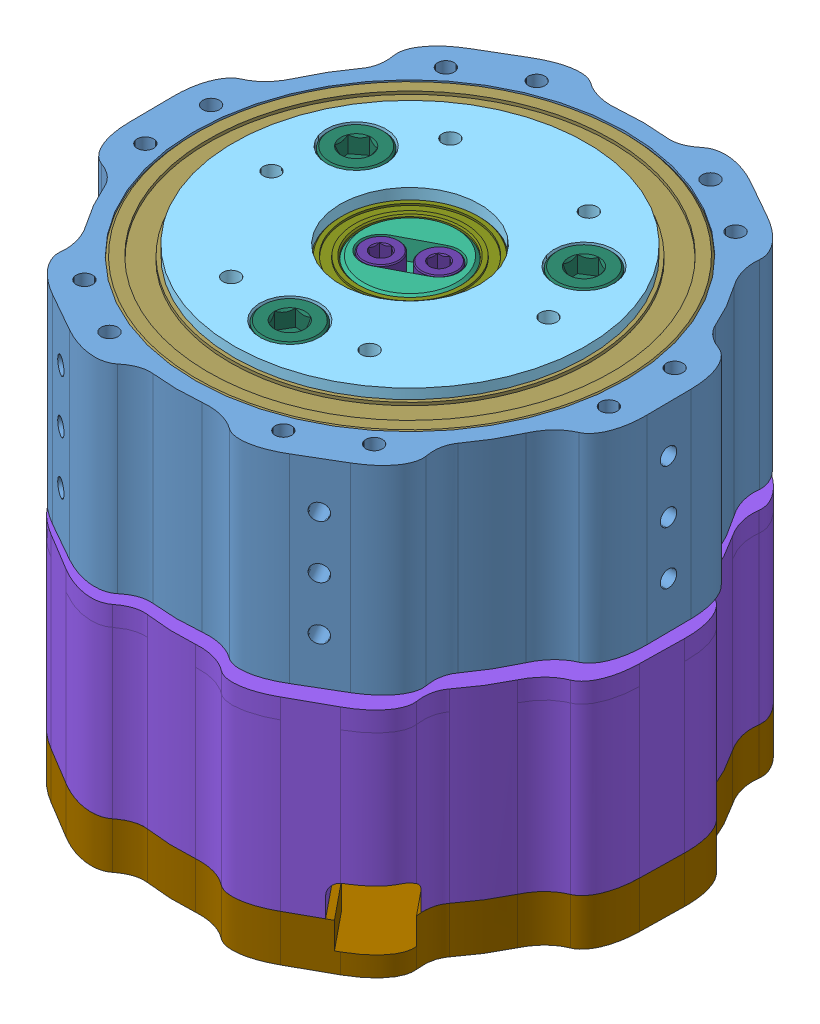
SolidWorks assembly LTRPT-0001-0000-00 (Assembly), configuration Resin 3D Print Config. Lengths in mm.
Overall size (104.8 68.77 105.06).
52 component instances, 20 part files, 70 mates.
Components (placement in the parent):
- LTRPT-0001-0001-00-1: LTRPT-0001-0001-00 [Pinless] at (0.2542 76.0347 0.3117) x (-0.492208 0 0.870478) z (-0.870478 0 -0.492208)
- LTRPT-0001-0002-00-1: LTRPT-0001-0002-00 [Default] at (0.2542 73.0347 0.3117) x (0.886253 0 -0.463201) z (0.463201 0 0.886253) (hidden)
- LTRPT-0001-0003-00-1: LTRPT-0001-0003-00 [Default] at (-0.632 82.5347 0.7749) x (-0.034899 0 -0.999391) z (0.999391 0 -0.034899)
- LTRPT-0001-0004-00-1: LTRPT-0001-0004-00 [Default] at (1.1405 91.5347 -0.1515) x (0.121869 0 -0.992546) z (0.992546 0 0.121869)
- LTRPT-0001-0005-00-1: LTRPT-0001-0005-00 [Default] at (0.2542 76.0347 0.3117) x (-0.998988 0 0.044987) z (-0.044987 0 -0.998988)
- LTRPT-0001-0006-00-1: LTRPT-0001-0006-00 [Default] at (0.2542 100.0347 0.3117) x (0.538454 0 0.842655) z (-0.842655 0 0.538454)
- LTRPT-0001-0007-00-1: LTRPT-0001-0007-00 [Default] at (1.1405 91.0347 -0.1515) x (-0.886253 0 0.463201) z (-0.463201 0 -0.886253)
- LTRPT-0001-0008-00-1: LTRPT-0001-0008-00 [Default] at (0.2542 76.0347 0.3117) x (-0.886253 0 0.463201) z (-0.463201 0 -0.886253)
- LTRPT-0001-0006-01-1: LTRPT-0001-0006-01 [Default] at (0.2542 100.0347 0.3117) x (0.538454 0 0.842655) z (-0.842655 0 0.538454) (hidden)
- LTRPT-0001-0009-00-1: LTRPT-0001-0009-00 [Pinless] at (0.2542 46.0347 0.3117) x (0.999837 0 0.018067) z (-0.018067 0 0.999837) size (77.35 28.07 76.65)
- LTRPT-0001-0010-01-1: LTRPT-0001-0010-01 [Default] at (0.2542 42.0347 0.3117) x (-0.999837 0 -0.018067) z (0 -1 0) size (77.35 73.91 7.07)
- LTRPT-0001-0011-00-1: LTRPT-0001-0011-00 [Default] at (0.2542 71.3347 0.3117) x (0.984702 0 0.174247) z (0 1 0) size (19.5 19.5 4.5)
- LTRPT-0001-0012-00-1: LTRPT-0001-0012-00 [Default] at (14.0653 40.3347 -2.5639) x (-0.953415 0 -0.301661) z (0 -1 0) size (77.35 73.91 4.57) (hidden)
- GARTT ML5008 330KV-1: GARTT ML5008 330KV [Default] at (0.2542 46.0347 0.3117) x (0.984702 0 0.174247) z (-0.174247 0 0.984702)
- 6656K229_Ultra-Thin Ball Bearing-1: 6656K229_Ultra-Thin Ball Bearing [6656K229] at (0.2542 102.5347 0.3117) x (0.90683 0 0.421496) z (0 1 0)
- 6656K229_Ultra-Thin Ball Bearing-2: 6656K229_Ultra-Thin Ball Bearing [6656K229] at (0.2542 79.5347 0.3117) x (0.89109 0 -0.453826) z (0 1 0)
- 5x25mm Dowel Pin-1: 5x25mm Dowel Pin [Default] at (-15.7562 78.0347 10.5424) x (-0.5743 0 0.818645) z (-0.818645 0 -0.5743)
- 5x25mm Dowel Pin-5: 5x25mm Dowel Pin [Default] at (17.1194 78.0347 9.0619) x (-0.146093 0 -0.989271) z (0.989271 0 -0.146093)
- 5x25mm Dowel Pin-6: 5x25mm Dowel Pin [Default] at (-0.6005 78.0347 -18.669) x (0.11323 0 -0.993569) z (0.993569 0 0.11323)
- MR95ZZ-1: MR95ZZ [Predeterminado] at (-15.7562 91.5347 10.5424) x (0.985719 0 -0.168399) z (0 1 0)
- MR95ZZ-2: MR95ZZ [Predeterminado] at (-15.7562 87.5347 10.5424) x (1 0 0.000798) z (0 1 0)
- MR95ZZ-3: MR95ZZ [Predeterminado] at (-15.7562 83.5347 10.5424) x (-0.502758 0 0.864427) z (0 1 0)
- MR95ZZ-4: MR95ZZ [Predeterminado] at (-15.7562 95.5347 10.5424) x (-0.758179 0 0.652046) z (0 1 0)
- 91290A252_Alloy Steel Socket Head Screw-1: 91290A252_Alloy Steel Socket Head Screw [Low Poly] at (16.2647 92.5347 -9.9189) x (0.999255 0 -0.038584) z (0 1 0)
- 91290A252_Alloy Steel Socket Head Screw-2: 91290A252_Alloy Steel Socket Head Screw [Low Poly] at (1.109 92.5347 19.2925) x (0.015336 0 -0.999882) z (0 1 0)
- 91290A252_Alloy Steel Socket Head Screw-3: 91290A252_Alloy Steel Socket Head Screw [Low Poly] at (-16.611 92.5347 -8.4384) x (-0.383105 0 0.923705) z (0 1 0)
- 6656K182_Ultra-Thin Ball Bearing-1: 6656K182_Ultra-Thin Ball Bearing [6656K182] at (0 79.0347 0) x (-0.858071 0 -0.513532) z (0 1 0)
- 6656K182_Ultra-Thin Ball Bearing-2: 6656K182_Ultra-Thin Ball Bearing [6656K182] at (0.2542 104.0347 0.3117) x (0.999223 0 -0.039404) z (0 1 0)
- 6656K182_Ultra-Thin Ball Bearing-3: 6656K182_Ultra-Thin Ball Bearing [6656K182] at (-0.632 88.0347 0.7749) x (0.999223 0 -0.039404) z (0 1 0)
- 6656K182_Ultra-Thin Ball Bearing-4: 6656K182_Ultra-Thin Ball Bearing [6656K182] at (1.1405 94.5347 -0.1515) x (0.999223 0 -0.039404) z (0 1 0)
- 91290A130_Black-Oxide Alloy Steel Socket Head Screw-1: 91290A130_Black-Oxide Alloy Steel Socket Head Screw [Low Poly] at (3.1345 89.5347 -1.1937) x (0.78846 0 0.615086) z (0 1 0)
- 91290A130_Black-Oxide Alloy Steel Socket Head Screw-2: 91290A130_Black-Oxide Alloy Steel Socket Head Screw [Low Poly] at (-2.6261 89.5347 1.8171) x (0.78846 0 0.615086) z (0 1 0)
- MR95ZZ-9: MR95ZZ [Predeterminado] at (-16.611 95.5347 -8.4384) x (-0.943778 0 -0.330579) z (0 1 0)
- MR95ZZ-10: MR95ZZ [Predeterminado] at (-0.6005 95.5347 -18.669) x (-0.185599 0 -0.982626) z (0 1 0)
- MR95ZZ-11: MR95ZZ [Predeterminado] at (16.2647 95.5347 -9.9189) x (0.758179 0 -0.652046) z (0 1 0)
- MR95ZZ-12: MR95ZZ [Predeterminado] at (17.1194 95.5347 9.0619) x (0.943778 0 0.330579) z (0 1 0)
- MR95ZZ-13: MR95ZZ [Predeterminado] at (1.109 95.5347 19.2925) x (0.185599 0 0.982626) z (0 1 0)
- MR95ZZ-14: MR95ZZ [Predeterminado] at (-16.611 91.5347 -8.4384) x (0.638697 0 0.769458) z (0 1 0)
- MR95ZZ-15: MR95ZZ [Predeterminado] at (-0.6005 91.5347 -18.669) x (-0.347022 0 0.937857) z (0 1 0)
- MR95ZZ-16: MR95ZZ [Predeterminado] at (16.2647 91.5347 -9.9189) x (-0.985719 0 0.168399) z (0 1 0)
- MR95ZZ-17: MR95ZZ [Predeterminado] at (17.1194 91.5347 9.0619) x (-0.638697 0 -0.769458) z (0 1 0)
- MR95ZZ-18: MR95ZZ [Predeterminado] at (1.109 91.5347 19.2925) x (0.347022 0 -0.937857) z (0 1 0)
- MR95ZZ-19: MR95ZZ [Predeterminado] at (-16.611 87.5347 -8.4384) x (0.499309 0 0.866424) z (0 1 0)
- MR95ZZ-20: MR95ZZ [Predeterminado] at (-0.6005 87.5347 -18.669) x (-0.500691 0 0.865626) z (0 1 0)
- MR95ZZ-21: MR95ZZ [Predeterminado] at (16.2647 87.5347 -9.9189) x (-1 0 -0.000798) z (0 1 0)
- MR95ZZ-22: MR95ZZ [Predeterminado] at (17.1194 87.5347 9.0619) x (-0.499309 0 -0.866424) z (0 1 0)
- MR95ZZ-23: MR95ZZ [Predeterminado] at (1.109 87.5347 19.2925) x (0.500691 0 -0.865626) z (0 1 0)
- MR95ZZ-24: MR95ZZ [Predeterminado] at (-16.611 83.5347 -8.4384) x (-0.999995 0 -0.003188) z (0 1 0)
- MR95ZZ-25: MR95ZZ [Predeterminado] at (-0.6005 83.5347 -18.669) x (-0.497237 0 -0.867615) z (0 1 0)
- MR95ZZ-26: MR95ZZ [Predeterminado] at (16.2647 83.5347 -9.9189) x (0.502758 0 -0.864427) z (0 1 0)
- MR95ZZ-27: MR95ZZ [Predeterminado] at (17.1194 83.5347 9.0619) x (0.999995 0 0.003188) z (0 1 0)
- MR95ZZ-28: MR95ZZ [Predeterminado] at (1.109 83.5347 19.2925) x (0.497237 0 0.867615) z (0 1 0)
Mates (geometry in assembly coordinates):
- Concentric5: concentric aligned: cylinder of Actuator Body-1 through (0.2542 0 0.3117) axis (0 -1 0) radius 35; cylinder of LTRPT-0001-0001-00-1 through (0.2542 84.0347 0.3117) axis (0 -1 0) radius 35
- Angle2: planar angle = 0.034907 rad anti-aligned: plane of LTRPT-0001-0003-00-1 through (-0.632 82.5347 0.7749) normal (-0.034899 0 -0.999391)
- Angle3: planar angle = 0.15708 rad aligned: plane of LTRPT-0001-0003-00-1 through (-0.632 82.5347 0.7749) normal (-0.034899 0 -0.999391); plane of LTRPT-0001-0004-00-1 through (1.1405 91.5347 -0.1515) normal (0.121869 0 -0.992546)
- Coincident27: coordinate: point of Eccentric Bottom Bearing Housing-1
- Concentric28: concentric aligned: cylinder of LTRPT-0001-0003-00-1 through (-0.632 90.5347 0.7749) axis (0 -1 0) radius 10.4; cylinder of LTRPT-0001-0008-00-1 through (-0.632 91.0347 0.7749) axis (0 -1 0) radius 7.5
- Coincident36: coincident aligned: plane of LTRPT-0001-0001-00-1 through (0.2542 84.0347 0.3117) normal (0 -1 0); plane of LTRPT-0001-0008-00-1 through (-0.632 84.0347 0.7749) normal (0 -1 0)
- Coincident37: coincident aligned: plane of LTRPT-0001-0001-00-1 through (0.2542 76.0347 0.3117) normal (0 -1 0); plane of 6656K229_Ultra-Thin Ball Bearing-2 through (-14.3363 76.0347 -28.3368) normal (0 -1 0)
- Coincident38: coincident aligned: plane of LTRPT-0001-0001-00-1 through (0.2542 106.0347 0.3117) normal (0 1 0); plane of 6656K229_Ultra-Thin Ball Bearing-1 through (13.8053 106.0347 -28.8429) normal (0 1 0)
- Concentric33: concentric anti-aligned: cylinder of LTRPT-0001-0006-00-1 through (-15.7562 100.0347 10.5424) axis (0 1 0) radius 2.5; cylinder of 5x25mm Dowel Pin-1 through (-15.7562 103.0347 10.5424) axis (0 -1 0) radius 2.5
- Concentric35: concentric anti-aligned: cylinder of LTRPT-0001-0006-00-1 through (-0.6005 100.0347 -18.669) axis (0 1 0) radius 2.5; cylinder of 5x25mm Dowel Pin-6 through (-0.6005 103.0347 -18.669) axis (0 -1 0) radius 2.5
- Concentric37: concentric anti-aligned: cylinder of LTRPT-0001-0006-00-1 through (17.1194 100.0347 9.0619) axis (0 1 0) radius 2.5; cylinder of 5x25mm Dowel Pin-5 through (17.1194 103.0347 9.0619) axis (0 -1 0) radius 2.5
- Concentric39: concentric anti-aligned: cylinder of 5x25mm Dowel Pin-1 through (-15.7562 103.0347 10.5424) axis (0 -1 0) radius 2.5; cylinder of MR95ZZ-1 through (-15.7562 91.5347 10.5424) axis (0 1 0) radius 2.5
- Concentric401: concentric aligned: cylinder of 5x25mm Dowel Pin-1 through (-15.7562 103.0347 10.5424) axis (0 -1 0) radius 2.5; cylinder of MR95ZZ-2 through (-15.7562 90.5347 10.5424) axis (0 -1 0) radius 4.5
- Concentric411: concentric aligned: cylinder of 5x25mm Dowel Pin-1 through (-15.7562 103.0347 10.5424) axis (0 -1 0) radius 2.5; cylinder of MR95ZZ-3 through (-15.7562 86.5347 10.5424) axis (0 -1 0) radius 4.5
- Concentric421: concentric aligned: cylinder of 5x25mm Dowel Pin-1 through (-15.7562 103.0347 10.5424) axis (0 -1 0) radius 2.5; cylinder of MR95ZZ-4 through (-15.7562 98.5347 10.5424) axis (0 -1 0) radius 4.5
- Distance1: distance = 1 mm anti-aligned: plane of MR95ZZ-2 through (-15.7562 87.5347 10.5424) normal (0 -1 0); plane of MR95ZZ-3 through (-15.7562 86.5347 10.5424) normal (0 1 0)
- Distance2: distance = 1 mm anti-aligned: plane of MR95ZZ-1 through (-15.7562 94.5347 10.5424) normal (0 1 0); plane of MR95ZZ-4 through (-15.7562 95.5347 10.5424) normal (0 -1 0)
- Concentric47: concentric anti-aligned: cylinder of LTRPT-0001-0006-00-1 through (1.109 100.0347 19.2925) axis (0 1 0) radius 2.5; cylinder of 91290A252_Alloy Steel Socket Head Screw-2 through (1.109 77.5347 19.2925) axis (0 -1 0) radius 4.25
- Concentric48: concentric anti-aligned: cylinder of LTRPT-0001-0006-00-1 through (-16.611 100.0347 -8.4384) axis (0 1 0) radius 2.5; cylinder of 91290A252_Alloy Steel Socket Head Screw-3 through (-16.611 77.5347 -8.4384) axis (0 -1 0) radius 4.25
- Coincident44: coincident aligned: plane of 6656K182_Ultra-Thin Ball Bearing-1 through (-5.2894 81.0347 8.8381) normal (0 1 0); circle of Inner Ring Base3DMETAL_EDIT-1
- Concentric57: concentric anti-aligned: cylinder of LTRPT-0001-0008-00-1 through (-0.632 91.0347 0.7749) axis (0 -1 0) radius 7.5; cylinder of 6656K182_Ultra-Thin Ball Bearing-3 through (-0.632 90.0347 0.7749) axis (0 1 0) radius 7.5
- Distance5: distance = 1 mm aligned: plane of 6656K182_Ultra-Thin Ball Bearing-3 through (-0.9604 90.0347 -7.5519) normal (0 1 0); plane of LTRPT-0001-0008-00-1 through (-0.632 91.0347 0.7749) normal (0 1 0)
- Coincident48: coincident aligned: plane of LTRPT-0001-0008-00-1 through (0.2542 76.0347 0.3117) normal (-0.463201 0 -0.886253); plane of LTRPT-0001-0007-00-1 through (1.1405 91.0347 -0.1515) normal (-0.463201 0 -0.886253)
- Concentric58: concentric aligned: cylinder of LTRPT-0001-0008-00-1 through (0.2542 84.0347 0.3117) axis (0 -1 0) radius 7.5; cylinder of LTRPT-0001-0007-00-1 through (0.2542 106.0347 0.3117) axis (0 -1 0) radius 7.5
- Concentric59: concentric anti-aligned: cylinder of LTRPT-0001-0004-00-1 through (1.1405 98.5347 -0.1515) axis (0 -1 0) radius 10.4; cylinder of 6656K182_Ultra-Thin Ball Bearing-4 through (1.1405 96.5347 -0.1515) axis (0 1 0) radius 7.5
- Distance6: distance = 1 mm aligned: plane of 6656K182_Ultra-Thin Ball Bearing-4 through (0.7346 92.5347 -10.4435) normal (0 -1 0); plane of LTRPT-0001-0004-00-1 through (-2.2113 91.5347 27.6478) normal (0 -1 0)
- Coincident50: coincident anti-aligned: plane of LTRPT-0001-0008-00-1 through (-0.632 91.0347 0.7749) normal (0 1 0); plane of LTRPT-0001-0007-00-1 through (1.1405 91.0347 -0.1515) normal (0 -1 0)
- Concentric60: concentric anti-aligned: cylinder of LTRPT-0001-0007-00-1 through (0.2542 106.0347 0.3117) axis (0 -1 0) radius 7.5; cylinder of 6656K182_Ultra-Thin Ball Bearing-2 through (0.2542 106.0347 0.3117) axis (0 1 0) radius 7.5
- Coincident51: coincident aligned: plane of LTRPT-0001-0007-00-1 through (0.2542 106.0347 0.3117) normal (0 1 0); plane of 6656K182_Ultra-Thin Ball Bearing-2 through (-0.0741 106.0347 -8.0151) normal (0 1 0)
- Coincident53: coincident anti-aligned: plane of LTRPT-0001-0001-00-1 through (0.2542 76.0347 0.3117) normal (0 -1 0); plane of LTRPT-0001-0005-00-1 through (0.2542 76.0347 0.3117) normal (0 1 0)
- Concentric64: concentric anti-aligned: cylinder of LTRPT-0001-0006-00-1 through (16.2647 100.0347 -9.9189) axis (0 1 0) radius 2.5; cylinder of 91290A252_Alloy Steel Socket Head Screw-1 through (16.2647 77.5347 -9.9189) axis (0 -1 0) radius 2.5
- Distance8: distance = 1 mm anti-aligned: plane of LTRPT-0001-0004-00-1 through (-2.2113 91.5347 27.6478) normal (0 -1 0); plane of LTRPT-0001-0003-00-1 through (0.4062 90.5347 28.7562) normal (0 1 0)
- Distance9: distance = 0.5 mm aligned: plane of LTRPT-0001-0008-00-1 through (-0.632 91.0347 0.7749) normal (0 1 0); plane of LTRPT-0001-0003-00-1 through (0.4062 90.5347 28.7562) normal (0 1 0)
- Distance10: distance = 1 mm anti-aligned: plane of MR95ZZ-1 through (-15.7562 91.5347 10.5424) normal (0 -1 0); plane of MR95ZZ-2 through (-15.7562 90.5347 10.5424) normal (0 1 0)
- Coincident57: coincident aligned: plane of 91290A252_Alloy Steel Socket Head Screw-1 through (16.1103 107.5347 -13.9159) normal (0 1 0); plane of 91290A252_Alloy Steel Socket Head Screw-2 through (-2.8905 107.5347 19.2312) normal (0 1 0)
- Coincident58: coincident aligned: plane of 91290A252_Alloy Steel Socket Head Screw-1 through (16.1103 107.5347 -13.9159) normal (0 1 0); plane of 91290A252_Alloy Steel Socket Head Screw-3 through (-12.9162 107.5347 -6.906) normal (0 1 0)
- Coincident59: coincident aligned: plane of 5x25mm Dowel Pin-5 through (17.1194 103.0347 9.0619) normal (0 1 0); plane of 5x25mm Dowel Pin-6 through (-0.6005 103.0347 -18.669) normal (0 1 0)
- Coincident60: coincident aligned: plane of 5x25mm Dowel Pin-1 through (-15.7562 103.0347 10.5424) normal (0 1 0); plane of 5x25mm Dowel Pin-5 through (17.1194 103.0347 9.0619) normal (0 1 0)
- Concentric67: concentric anti-aligned: cylinder of LTRPT-0001-0007-00-1 through (1.1405 99.0347 -0.1515) axis (0 -1 0) radius 7.5; cylinder of 6656K182_Ultra-Thin Ball Bearing-4 through (1.1405 96.5347 -0.1515) axis (0 1 0) radius 7.5
- Concentric69: concentric anti-aligned: circle of ECCENTRIC SHAFT-1; cylinder of LTRPT-0001-0002-00-1 through (3.1345 73.0347 -1.1937) axis (0 1 0) radius 1.25
- Coincident64: coincident anti-aligned: plane of LTRPT-0001-0008-00-1 through (0.2542 76.0347 0.3117) normal (0 -1 0); plane of LTRPT-0001-0002-00-1 through (0.2542 76.0347 0.3117) normal (0 1 0)
- Concentric70: concentric anti-aligned: cylinder of LTRPT-0001-0007-00-1 through (3.1345 91.0347 -1.1937) axis (0 1 0) radius 1.5; cylinder of 91290A130_Black-Oxide Alloy Steel Socket Head Screw-1 through (3.1345 73.0347 -1.1937) axis (0 -1 0) radius 1.5
- Concentric71: concentric anti-aligned: cylinder of LTRPT-0001-0007-00-1 through (-2.6261 91.0347 1.8171) axis (0 1 0) radius 1.5; cylinder of 91290A130_Black-Oxide Alloy Steel Socket Head Screw-2 through (-2.6261 73.0347 1.8171) axis (0 -1 0) radius 1.5
- Coincident65: coincident aligned: plane of 91290A130_Black-Oxide Alloy Steel Socket Head Screw-1 through (3.1345 106.0347 -1.1937) normal (0 1 0); plane of 91290A130_Black-Oxide Alloy Steel Socket Head Screw-2 through (-2.6261 106.0347 1.8171) normal (0 1 0)
- Coincident66: coincident anti-aligned: plane of LTRPT-0001-0007-00-1 through (3.1345 103.0347 -1.1937) normal (0 1 0); plane of 91290A130_Black-Oxide Alloy Steel Socket Head Screw-2 through (-1.0269 103.0347 -0.2328) normal (0 -1 0)
- Coincident68: coincident anti-aligned: plane of LTRPT-0001-0006-00-1 through (1.109 102.5347 19.2925) normal (0 1 0); plane of 91290A252_Alloy Steel Socket Head Screw-2 through (1.0476 102.5347 23.292) normal (0 -1 0)
- Coincident69: coincident anti-aligned: plane of LTRPT-0001-0006-00-1 through (17.1194 103.0347 9.0619) normal (0 -1 0); plane of 5x25mm Dowel Pin-5 through (17.1194 103.0347 9.0619) normal (0 1 0)
- Concentric72: concentric anti-aligned: cylinder of LTRPT-0001-0005-00-1 through (16.2647 76.0347 -9.9189) axis (0 1 0) radius 2.15; cylinder of 91290A252_Alloy Steel Socket Head Screw-1 through (16.2647 77.5347 -9.9189) axis (0 -1 0) radius 2.5
- Coincident70: coincident anti-aligned: plane of LTRPT-0001-0006-00-1 through (0.2542 106.0347 0.3117) normal (0 -1 0); plane of 6656K229_Ultra-Thin Ball Bearing-1 through (13.8053 106.0347 -28.8429) normal (0 1 0)
- Coincident71: coincident aligned: plane of LTRPT-0001-0003-00-1 through (0.4062 90.5347 28.7562) normal (0 1 0); plane of MR95ZZ-2 through (-15.7562 90.5347 10.5424) normal (0 1 0)
- Concentric422: concentric aligned: cylinder of LTRPT-0001-0006-00-1 through (0.2542 106.0347 0.3117) axis (0 -1 0) radius 25; cylinder of LTRPT-0001-0001-00-1 through (0.2542 106.0347 0.3117) axis (0 -1 0) radius 32.5
- Concentric423: concentric anti-aligned: cylinder of LTRPT-0001-0001-00-1 through (0.2542 84.0347 0.3117) axis (0 -1 0) radius 32.5; cylinder of 6656K229_Ultra-Thin Ball Bearing-2 through (0.2542 83.0347 0.3117) axis (0 1 0) radius 32.5
- Concentric424: concentric anti-aligned: cylinder of LTRPT-0001-0005-00-1 through (0.2542 82.0347 0.3117) axis (0 -1 0) radius 10.5; cylinder of 6656K229_Ultra-Thin Ball Bearing-2 through (0.2542 83.0347 0.3117) axis (0 1 0) radius 25
- Concentric425: concentric anti-aligned: cylinder of LTRPT-0001-0001-00-1 through (0.2542 84.0347 0.3117) axis (0 -1 0) radius 32.5; cylinder of LTRPT-0001-0002-00-1 through (0.2542 70.0347 0.3117) axis (0 1 0) radius 15
- Concentric426: concentric anti-aligned: cylinder of LTRPT-0001-0001-00-1 through (0.2542 106.0347 0.3117) axis (0 -1 0) radius 32.5; cylinder of 6656K229_Ultra-Thin Ball Bearing-1 through (0.2542 106.0347 0.3117) axis (0 1 0) radius 32.5
- Concentric427: concentric aligned: cylinder of LTRPT-0001-0006-00-1 through (0.2542 100.0337 0.3117) axis (0 1 0) radius 10.5; cylinder of 6656K182_Ultra-Thin Ball Bearing-2 through (0.2542 106.0347 0.3117) axis (0 1 0) radius 10.5
- Coincident73: coincident anti-aligned: plane of LTRPT-0001-0001-00-1 through (0.2542 106.0347 0.3117) normal (0 1 0); plane of LTRPT-0001-0006-01-1 through (0.2542 106.0347 0.3117) normal (0 -1 0)
- Concentric429: concentric anti-aligned: cylinder of 6656K229_Ultra-Thin Ball Bearing-1 through (0.2542 106.0347 0.3117) axis (0 1 0) radius 25; cylinder of LTRPT-0001-0006-01-1 through (0.2542 106.0347 0.3117) axis (0 -1 0) radius 25
- Concentric430: concentric anti-aligned: cylinder of GARTT ML5008 330KV-1 through (0.2542 71.3347 0.3117) axis (0 -1 0) radius 29.5; cylinder of LTRPT-0001-0002-00-1 through (0.2542 70.0347 0.3117) axis (0 1 0) radius 15
- Concentric431: concentric aligned: cylinder of GARTT ML5008 330KV-1 through (0.2542 71.3347 0.3117) axis (0 -1 0) radius 29.5; cylinder of LTRPT-0001-0009-00-1 through (0.2542 63.0347 0.3117) axis (0 -1 0) radius 32.5
- Parallel1: parallel anti-aligned: cylinder of LTRPT-0001-0005-00-1 through (-8.9579 79.0347 18.0655) axis (0 -1 0) radius 1.25; cylinder of LTRPT-0001-0009-00-1 through (20.251 74.0713 0.6731) axis (0 1 0) radius 1.5
- Coincident74: coincident aligned: plane of GARTT ML5008 330KV-1 through (0.2542 46.0347 0.3117) normal (0 -1 0); plane of LTRPT-0001-0009-00-1 through (0.2542 46.0347 0.3117) normal (0 -1 0)
- Coincident78: coincident anti-aligned: plane of LTRPT-0001-0005-00-1 through (0.2542 74.0347 0.3117) normal (0 -1 0); plane of LTRPT-0001-0009-00-1 through (28.009 74.0347 -21.9323) normal (0 1 0)
- InPlace2: in place: plane of GARTT ML5008 330KV-1 through (0.2542 71.3347 0.3117) normal (0 1 0); plane of ? through (0 71.3347 0) normal (0 1 0); moOrthogonalPlaneRef_w of GARTT ML5008 330KV-1 through (0.2542 71.3347 0.3117) normal (0 1 0); plane of ? through (0 71.3347 0) normal (0 0 -1); plane of GARTT ML5008 330KV-1 through (0.2542 71.3347 0.3117) normal (0 1 0); plane of ? through (0 71.3347 0) normal (1 0 0); plane of GARTT ML5008 330KV-1 through (0.2542 71.3347 0.3117) normal (0 1 0); unknown of LTRPT-0001-0011-00-1
- Coincident79: coincident aligned: plane of GARTT ML5008 330KV-1; plane of LTRPT-0001-0011-00-1
- Coincident80: coincident aligned: moOrthogonalPlaneRef_w of GARTT ML5008 330KV-1 through (0.2542 71.3347 0.3117) normal (0.174247 0 -0.984702); plane of LTRPT-0001-0011-00-1 through (0.2542 71.3347 0.3117) normal (0.174247 0 -0.984702)
- Coincident81: coincident anti-aligned: moOrthogonalPlaneRef_w of GARTT ML5008 330KV-1 through (0.2542 71.3347 0.3117) normal (-0.984702 0 -0.174247); plane of LTRPT-0001-0011-00-1 through (0.2542 71.3347 0.3117) normal (0.984702 0 0.174247)
- Coincident79: coincident anti-aligned: plane of LTRPT-0001-0009-00-1 through (0.2542 46.0347 0.3117) normal (0 -1 0); plane of LTRPT-0001-0010-01-1 through (25.3433 46.0347 29.866) normal (0 1 0)
- Coincident80: coincident aligned: circle of LTRPT-0001-0009-00-1; cylinder of LTRPT-0001-0010-01-1 through (-20.896 39.0347 -27.5749) axis (0 1 0) radius 1.25
- Concentric432: concentric anti-aligned: circle of LTRPT-0001-0009-00-1; circle of LTRPT-0001-0010-01-1
